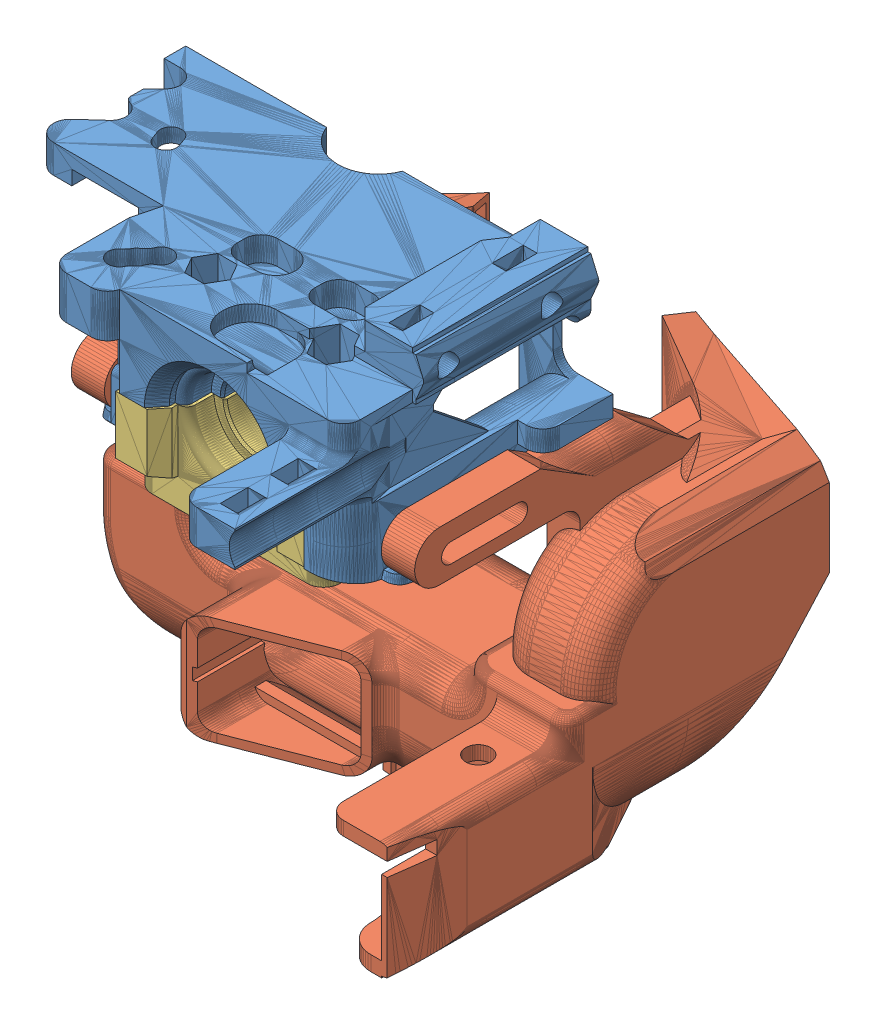
SolidWorks assembly Assem2, configuration Default. Lengths in mm.
Overall size (90.08 84.53 89.37).
3 component instances, 3 part files, 6 mates.
Components (placement in the parent):
- BB_M.Base_2.7.21.-1: BB_M.Base_2.7.21. [Default] at (-24.6902 -13.5646 2.1923) size (76.99 37.19 63.54)
- Untitled.step-1: Untitled.step [Default] at (-22.931 -24.815 -10.126) size (85.26 60.11 77.93)
- BB_M.Cap_2.7.21-1: BB_M.Cap_2.7.21 [Default] at (-24.1902 -13.2975 2.192) size (33.92 16.28 16.79)
Mates (geometry in assembly coordinates):
- Coincident7: coincident anti-aligned: plane of BB_M.Base_2.7.21.-1 through (5.7871 -13.5646 2.1923) normal (1 0 0); plane of Untitled.step-1 through (5.7871 -11.7391 -29.5435) normal (-1 0 0)
- Coincident8: coincident anti-aligned: plane of BB_M.Base_2.7.21.-1 through (-24.6902 -3.7391 2.1923) normal (0 -1 0); plane of Untitled.step-1 through (11.7951 -3.7391 14.3463) normal (0 1 0)
- Lock1: lock: unknown of BB_M.Base_2.7.21.-1; unknown of Untitled.step-1
- Coincident10: coincident: plane of BB_M.Base_2.7.21.-1 through (-24.6902 -0.465 2.1923) normal (0 -1 0); plane of BB_M.Cap_2.7.21-1 through (-24.1902 -0.465 5.7423) normal (0 1 0)
- Coincident11: coincident: plane of BB_M.Base_2.7.21.-1 through (-1.4192 -13.5646 2.1923) normal (-1 0 0); plane of BB_M.Cap_2.7.21-1 through (-1.4192 -13.2975 5.7423) normal (1 0 0)
- Coincident13: coincident aligned: plane of BB_M.Base_2.7.21.-1 through (-24.6902 -13.5646 25.5845) normal (0 0 1); plane of BB_M.Cap_2.7.21-1 through (-24.1902 -13.2975 25.5845) normal (0 0 1)
